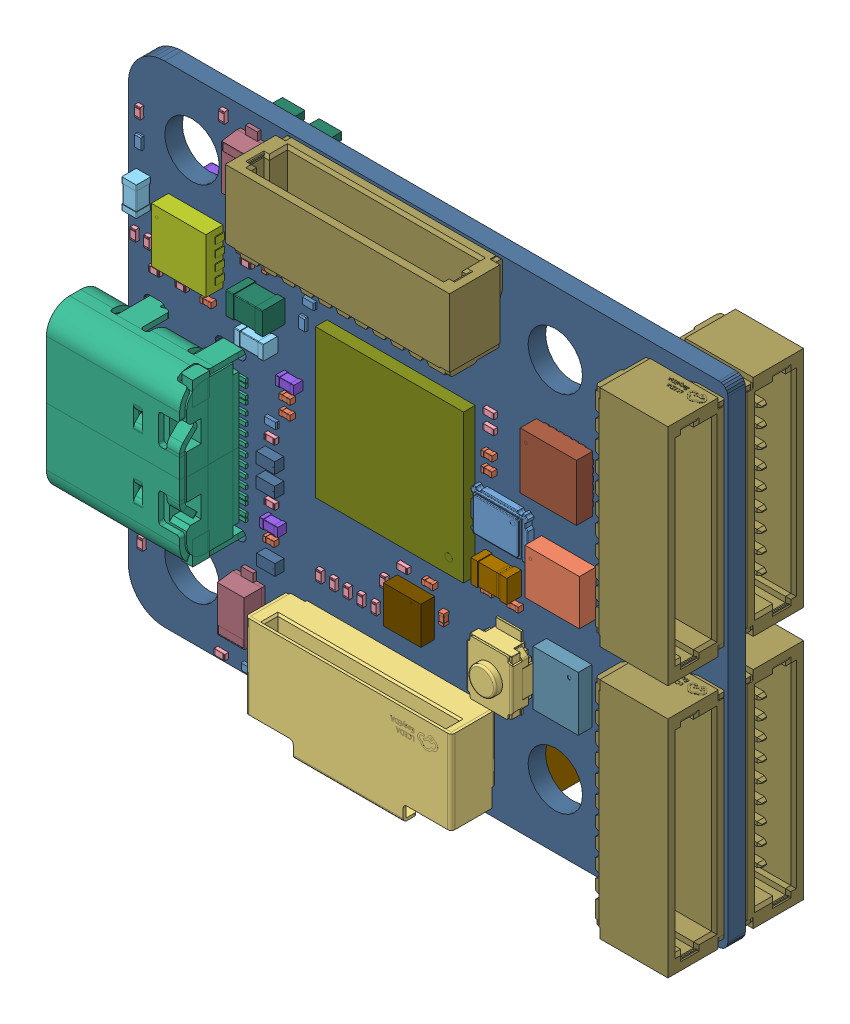
SolidWorks assembly NxtPX4, configuration 默认. Lengths in mm.
Overall size (34.16 27.21 7.57).
256 component instances, 28 part files, 0 mates.
Components (placement in the parent):
- NxtPX4.step-1: NxtPX4.step [默认] at origin size (34.16 27.21 7.57)
  - LED_0201_0603Metric.step-1: LED_0201_0603Metric.step [默认] at (3.0707 13.3273 1.012) x (-1 0 0) z (0 0 1) size (0.65 0.35 0.2)
    - SOLID.step-1: SOLID.step [默认] at origin size (0.65 0.35 0.2)
  - C_0201_0603Metric.step-1: C_0201_0603Metric.step [默认] at (-0.3793 17.3773 1.012) size (0.6 0.3 0.3)
    - SOLID-0.step-1: SOLID-0.step [默认] at origin size (0.6 0.3 0.3)
  - C_0201_0603Metric.step-2: C_0201_0603Metric.step [默认] at (15.0907 17.8073 1.012) size (0.6 0.3 0.3)
    - SOLID-0.step-1: SOLID-0.step [默认] at origin size (0.6 0.3 0.3)
  - C_0201_0603Metric.step-3: C_0201_0603Metric.step [默认] at (15.0707 11.3173 1.012) size (0.6 0.3 0.3)
    - SOLID-0.step-1: SOLID-0.step [默认] at origin size (0.6 0.3 0.3)
  - SW_SPST_B3U-1000P-B.step-1: SW_SPST_B3U-1000P-B.step [默认] at (16.1107 8.1973 1.012) x (0 1 0) z (0 0 1) size (4 2.51 2.09)
    - SOLID-1.step-1: SOLID-1.step [默认] at origin size (4 2.51 2.09)
  - R_0201_0603Metric.step-1: R_0201_0603Metric.step [默认] at (9.2907 8.8573 1.012) x (0 -1 0) z (0 0 1) size (0.6 0.3 0.23)
    - SOLID-2.step-1: SOLID-2.step [默认] at origin size (0.6 0.3 0.23)
  - LED_0201_0603Metric.step-2: LED_0201_0603Metric.step [默认] at (4.8107 18.9173 1.012) x (0 1 0) z (0 0 1) size (0.65 0.35 0.2)
    - SOLID.step-1: SOLID.step [默认] at origin size (0.65 0.35 0.2)
  - C_0603_1608Metric.step-1: C_0603_1608Metric.step [默认] at (2.5007 17.0773 1.012) size (1.6 0.8 0.8)
    - SOLID-3.step-1: SOLID-3.step [默认] at origin size (1.6 0.8 0.8)
  - USB_C_Receptacle_GCT_USB4105-xx-A_16P_TopMnt_Horizontal.step-1: USB_C_Receptacle_GCT_USB4105-xx-A_16P_TopMnt_Horizontal.step [默认] at (-2.4493 11.2373 1.012) x (0 -1 0) z (0 0 1) size (8.94 7.78 4.26)
    - COMPOUND.step-1: COMPOUND.step [默认] at origin size (8.94 7.78 4.26)
  - QFN8_3X3_MPS.step-1: QFN8_3X3_MPS.step [默认] at (-1.1693 19.8273 1.012) size (3.1 3 1)
    - COMPOUND-4.step-1: COMPOUND-4.step [默认] at origin size (3.1 3 1)
  - C_0603_1608Metric.step-2: C_0603_1608Metric.step [默认] at (-4.0893 20.7873 1.012) x (0 1 0) z (0 0 1) size (1.6 0.8 0.8)
    - SOLID-3.step-1: SOLID-3.step [默认] at origin size (1.6 0.8 0.8)
  - LED_0201_0603Metric.step-3: LED_0201_0603Metric.step [默认] at (5.1607 20.0473 1.012) size (0.65 0.35 0.2)
    - SOLID.step-1: SOLID.step [默认] at origin size (0.65 0.35 0.2)
  - R_0201_0603Metric.step-2: R_0201_0603Metric.step [默认] at (0.4307 26.6173 1.012) x (0 1 0) z (0 0 1) size (0.6 0.3 0.23)
    - SOLID-2.step-1: SOLID-2.step [默认] at origin size (0.6 0.3 0.23)
  - C_0402_1005Metric.step-1: C_0402_1005Metric.step [默认] at (4.1807 15.8173 1.012) x (-1 0 0) z (0 0 1) size (1 0.5 0.5)
    - SOLID-5.step-1: SOLID-5.step [默认] at origin size (1 0.5 0.5)
  - CAP_ABS07-32_768KHZ-T_ABR.step-1: CAP_ABS07-32_768KHZ-T_ABR.step [默认] at (15.7207 12.4073 1.012) x (-1 0 0) z (0 0 1) size (1.98 1.26 0.8)
    - COMPOUND-6.step-1: COMPOUND-6.step [默认] at origin size (1.98 1.26 0.8)
  - DFN1006-2_SOD882_NEX.step-1: DFN1006-2_SOD882_NEX.step [默认] at (3.1307 10.4373 1.012) x (-1 0 0) z (0 0 1) size (1.02 0.61 0.51)
    - COMPOUND-7.step-1: COMPOUND-7.step [默认] at origin size (1.02 0.61 0.51)
  - QFN24_3X3X0P9_IVS_ICM20649.step-1: QFN24_3X3X0P9_IVS_ICM20649.step [默认] at (19.1391 19.1673 1.012) size (3.1 3.1 0.94)
    - COMPOUND-8.step-1: COMPOUND-8.step [默认] at origin size (3.1 3.1 0.94)
  - C_0201_0603Metric.step-4: C_0201_0603Metric.step [默认] at (15.0807 17.0373 1.012) size (0.6 0.3 0.3)
    - SOLID-0.step-1: SOLID-0.step [默认] at origin size (0.6 0.3 0.3)
  - sh1.0_10P.step-1: sh1.0_10P.step [默认] at (9.7807 24.6273 1.012) x (-1 0 0) z (0 0 1) size (12.36 5 3.2)
    - COMPOUND-9.step-1: COMPOUND-9.step [默认] at origin size (12.36 5 3.2)
  - D_SOD-123F.step-1: D_SOD-123F.step [默认] at (2.0507 25.0998 1.012) x (0 -1 0) z (0 0 1) size (3.5 1.6 1.1)
    - SOLID-10.step-1: SOLID-10.step [默认] at origin size (3.5 1.6 1.1)
  - R_0201_0603Metric.step-3: R_0201_0603Metric.step [默认] at (-4.4593 18.5473 1.012) x (0 -1 0) z (0 0 1) size (0.6 0.3 0.23)
    - SOLID-2.step-1: SOLID-2.step [默认] at origin size (0.6 0.3 0.23)
  - LED_0201_0603Metric.step-4: LED_0201_0603Metric.step [默认] at (5.1607 20.8073 1.012) size (0.65 0.35 0.2)
    - SOLID.step-1: SOLID.step [默认] at origin size (0.65 0.35 0.2)
  - R_0201_0603Metric.step-4: R_0201_0603Metric.step [默认] at (3.0707 9.4673 1.012) x (-1 0 0) z (0 0 1) size (0.6 0.3 0.23)
    - SOLID-2.step-1: SOLID-2.step [默认] at origin size (0.6 0.3 0.23)
  - R_0201_0603Metric.step-5: R_0201_0603Metric.step [默认] at (-4.0793 4.0023 1.012) x (0 1 0) z (0 0 1) size (0.6 0.3 0.23)
    - SOLID-2.step-1: SOLID-2.step [默认] at origin size (0.6 0.3 0.23)
  - C_0201_0603Metric.step-5: C_0201_0603Metric.step [默认] at (3.9707 14.9473 1.012) x (-1 0 0) z (0 0 1) size (0.6 0.3 0.3)
    - SOLID-0.step-1: SOLID-0.step [默认] at origin size (0.6 0.3 0.3)
  - R_0201_0603Metric.step-6: R_0201_0603Metric.step [默认] at (5.7607 7.3673 1.012) x (0 1 0) z (0 0 1) size (0.6 0.3 0.23)
    - SOLID-2.step-1: SOLID-2.step [默认] at origin size (0.6 0.3 0.23)
  - LGA-14_3x2.5mm_P0.5mm_LayoutBorder3x4y.step-1: LGA-14_3x2.5mm_P0.5mm_LayoutBorder3x4y.step [默认] at (19.3757 8.9973 1.012) x (0 -1 0) z (0 0 1) size (3 2.5 0.78)
    - SOLID-11.step-1: SOLID-11.step [默认] at origin size (3 2.5 0.78)
  - R_0201_0603Metric.step-7: R_0201_0603Metric.step [默认] at (15.1207 19.0473 1.012) size (0.6 0.3 0.23)
    - SOLID-2.step-1: SOLID-2.step [默认] at origin size (0.6 0.3 0.23)
  - C_0805_2012Metric.step-1: C_0805_2012Metric.step [默认] at (2.7007 18.8773 1.012) size (2 1.25 1.25)
    - SOLID-12.step-1: SOLID-12.step [默认] at origin size (2 1.25 1.25)
  - C_0201_0603Metric.step-6: C_0201_0603Metric.step [默认] at (11.8257 10.0373 1.012) x (-1 0 0) z (0 0 1) size (0.6 0.3 0.3)
    - SOLID-0.step-1: SOLID-0.step [默认] at origin size (0.6 0.3 0.3)
  - R_0201_0603Metric.step-8: R_0201_0603Metric.step [默认] at (23.1807 13.9673 1.012) x (-1 0 0) z (0 0 1) size (0.6 0.3 0.23)
    - SOLID-2.step-1: SOLID-2.step [默认] at origin size (0.6 0.3 0.23)
  - C_0201_0603Metric.step-7: C_0201_0603Metric.step [默认] at (2.8507 20.6773 1.012) x (0 -1 0) z (0 0 1) size (0.6 0.3 0.3)
    - SOLID-0.step-1: SOLID-0.step [默认] at origin size (0.6 0.3 0.3)
  - R_0201_0603Metric.step-9: R_0201_0603Metric.step [默认] at (3.0707 12.5673 1.012) x (-1 0 0) z (0 0 1) size (0.6 0.3 0.23)
    - SOLID-2.step-1: SOLID-2.step [默认] at origin size (0.6 0.3 0.23)
  - sh1.0_10P.step-2: sh1.0_10P.step [默认] at (25.1807 20.9273 1.012) x (0 1 0) z (0 0 1) size (12.36 5 3.2)
    - COMPOUND-9.step-1: COMPOUND-9.step [默认] at origin size (12.36 5 3.2)
  - TFBGA100.step-1: TFBGA100.step [默认] at (10.0407 15.4873 0.512) x (-1 0 0) z (0 0 1) size (8.15 8.15 1.1)
    - COMPOUND-13.step-1: COMPOUND-13.step [默认] at origin size (8.15 8.15 1.1)
  - R_0201_0603Metric.step-10: R_0201_0603Metric.step [默认] at (15.1207 19.8073 1.012) x (-1 0 0) z (0 0 1) size (0.6 0.3 0.23)
    - SOLID-2.step-1: SOLID-2.step [默认] at origin size (0.6 0.3 0.23)
  - LED_0201_0603Metric.step-5: LED_0201_0603Metric.step [默认] at (-4.2093 23.0523 1.012) x (0 -1 0) z (0 0 1) size (0.65 0.35 0.2)
    - SOLID.step-1: SOLID.step [默认] at origin size (0.65 0.35 0.2)
  - R_0201_0603Metric.step-11: R_0201_0603Metric.step [默认] at (-3.6993 18.5473 1.012) x (0 -1 0) z (0 0 1) size (0.6 0.3 0.23)
    - SOLID-2.step-1: SOLID-2.step [默认] at origin size (0.6 0.3 0.23)
  - D_SOD-123F.step-2: D_SOD-123F.step [默认] at (1.8107 3.9373 1.012) x (0 1 0) z (0 0 1) size (3.5 1.6 1.1)
    - SOLID-10.step-1: SOLID-10.step [默认] at origin size (3.5 1.6 1.1)
  - D_SOD-523.step-1: D_SOD-523.step [默认] at (1.9607 22.1373 1.012) size (1.6 0.8 0.63)
    - SOLID-14.step-1: SOLID-14.step [默认] at origin size (1.6 0.8 0.63)
  - R_0201_0603Metric.step-12: R_0201_0603Metric.step [默认] at (8.8007 7.3673 1.012) x (0 1 0) z (0 0 1) size (0.6 0.3 0.23)
    - SOLID-2.step-1: SOLID-2.step [默认] at origin size (0.6 0.3 0.23)
  - sh1.0_10P.step-3: sh1.0_10P.step [默认] at (25.1807 6.9973 1.012) x (0 1 0) z (0 0 1) size (12.36 5 3.2)
    - COMPOUND-9.step-1: COMPOUND-9.step [默认] at origin size (12.36 5 3.2)
  - DFN1006-2_SOD882_NEX.step-2: DFN1006-2_SOD882_NEX.step [默认] at (3.1307 11.6073 1.012) x (-1 0 0) z (0 0 1) size (1.02 0.61 0.51)
    - COMPOUND-7.step-1: COMPOUND-7.step [默认] at origin size (1.02 0.61 0.51)
  - R_0201_0603Metric.step-13: R_0201_0603Metric.step [默认] at (-3.3093 17.3873 1.012) size (0.6 0.3 0.23)
    - SOLID-2.step-1: SOLID-2.step [默认] at origin size (0.6 0.3 0.23)
  - C_0201_0603Metric.step-8: C_0201_0603Metric.step [默认] at (3.0807 7.7273 1.012) size (0.6 0.3 0.3)
    - SOLID-0.step-1: SOLID-0.step [默认] at origin size (0.6 0.3 0.3)
  - C_0201_0603Metric.step-9: C_0201_0603Metric.step [默认] at (12.5807 8.7773 1.012) x (0 -1 0) z (0 0 1) size (0.6 0.3 0.3)
    - SOLID-0.step-1: SOLID-0.step [默认] at origin size (0.6 0.3 0.3)
  - QFN_BMP388_BOS.step-1: QFN_BMP388_BOS.step [默认] at (10.9607 8.4148 1.012) x (0 -1 0) z (0 0 1) size (2.06 2.06 0.82)
    - COMPOUND-15.step-1: COMPOUND-15.step [默认] at origin size (2.06 2.06 0.82)
  - R_0201_0603Metric.step-14: R_0201_0603Metric.step [默认] at (24.6607 13.9673 1.012) size (0.6 0.3 0.23)
    - SOLID-2.step-1: SOLID-2.step [默认] at origin size (0.6 0.3 0.23)
  - C_0402_1005Metric.step-2: C_0402_1005Metric.step [默认] at (3.2907 8.5973 1.012) size (1 0.5 0.5)
    - SOLID-5.step-1: SOLID-5.step [默认] at origin size (1 0.5 0.5)
  - R_0201_0603Metric.step-15: R_0201_0603Metric.step [默认] at (0.3157 0.9173 1.012) size (0.6 0.3 0.23)
    - SOLID-2.step-1: SOLID-2.step [默认] at origin size (0.6 0.3 0.23)
  - R_0201_0603Metric.step-16: R_0201_0603Metric.step [默认] at (8.0407 7.3673 1.012) x (0 1 0) z (0 0 1) size (0.6 0.3 0.23)
    - SOLID-2.step-1: SOLID-2.step [默认] at origin size (0.6 0.3 0.23)
  - Oscillator_SMD_Abracon_ASV-4Pin_7.0x5.1mm.step-1: Oscillator_SMD_Abracon_ASV-4Pin_7.0x5.1mm.step [默认] at (15.8307 14.9373 1.012) x (-1 0 0) z (0 0 1) size (3.15 2.29 0.55)
    - COMPOUND-16.step-1: COMPOUND-16.step [默认] at origin size (3.15 2.29 0.55)
  - R_0201_0603Metric.step-17: R_0201_0603Metric.step [默认] at (7.2807 7.3673 1.012) x (0 1 0) z (0 0 1) size (0.6 0.3 0.23)
    - SOLID-2.step-1: SOLID-2.step [默认] at origin size (0.6 0.3 0.23)
  - R_0201_0603Metric.step-18: R_0201_0603Metric.step [默认] at (1.7307 21.0273 1.012) size (0.6 0.3 0.23)
    - SOLID-2.step-1: SOLID-2.step [默认] at origin size (0.6 0.3 0.23)
  - R_0201_0603Metric.step-19: R_0201_0603Metric.step [默认] at (10.3607 10.0373 1.012) x (-1 0 0) z (0 0 1) size (0.6 0.3 0.23)
    - SOLID-2.step-1: SOLID-2.step [默认] at origin size (0.6 0.3 0.23)
  - LED_0201_0603Metric.step-6: LED_0201_0603Metric.step [默认] at (1.7907 0.9173 1.012) size (0.65 0.35 0.2)
    - SOLID.step-1: SOLID.step [默认] at origin size (0.65 0.35 0.2)
  - C_0201_0603Metric.step-10: C_0201_0603Metric.step [默认] at (3.9707 14.1873 1.012) x (-1 0 0) z (0 0 1) size (0.6 0.3 0.3)
    - SOLID-0.step-1: SOLID-0.step [默认] at origin size (0.6 0.3 0.3)
  - R_0201_0603Metric.step-20: R_0201_0603Metric.step [默认] at (1.7307 20.2673 1.012) x (-1 0 0) z (0 0 1) size (0.6 0.3 0.23)
    - SOLID-2.step-1: SOLID-2.step [默认] at origin size (0.6 0.3 0.23)
  - R_0201_0603Metric.step-21: R_0201_0603Metric.step [默认] at (-1.8493 17.3773 1.012) size (0.6 0.3 0.23)
    - SOLID-2.step-1: SOLID-2.step [默认] at origin size (0.6 0.3 0.23)
  - R_0201_0603Metric.step-22: R_0201_0603Metric.step [默认] at (-4.2093 24.5023 1.012) x (0 -1 0) z (0 0 1) size (0.6 0.3 0.23)
    - SOLID-2.step-1: SOLID-2.step [默认] at origin size (0.6 0.3 0.23)
  - LGA14_2P5X3X0P91_IVS_ICM42688-P.step-1: LGA14_2P5X3X0P91_IVS_ICM42688-P.step [默认] at (19.3707 14.0373 1.012) size (3 2.49 0.97)
    - COMPOUND-17.step-1: COMPOUND-17.step [默认] at origin size (3 2.49 0.97)
  - LED_0201_0603Metric.step-7: LED_0201_0603Metric.step [默认] at (-4.0793 5.4598 1.012) x (0 1 0) z (0 0 1) size (0.65 0.35 0.2)
    - SOLID.step-1: SOLID.step [默认] at origin size (0.65 0.35 0.2)
  - R_0201_0603Metric.step-23: R_0201_0603Metric.step [默认] at (6.5207 7.3673 1.012) x (0 1 0) z (0 0 1) size (0.6 0.3 0.23)
    - SOLID-2.step-1: SOLID-2.step [默认] at origin size (0.6 0.3 0.23)
  - C_0201_0603Metric.step-11: C_0201_0603Metric.step [默认] at (16.5307 11.3173 1.012) x (-1 0 0) z (0 0 1) size (0.6 0.3 0.3)
    - SOLID-0.step-1: SOLID-0.step [默认] at origin size (0.6 0.3 0.3)
  - sd_card.step-1: sd_card.step [默认] at (9.9307 2.6273 1.012) x (-1 0 0) z (0 0 1) size (11.35 5.5 2.5)
    - COMPOUND-18.step-1: COMPOUND-18.step [默认] at origin size (11.35 5.5 2.5)
  - R_0201_0603Metric.step-24: R_0201_0603Metric.step [默认] at (3.6407 20.8673 1.012) x (0 -1 0) z (0 0 1) size (0.6 0.3 0.23)
    - SOLID-2.step-1: SOLID-2.step [默认] at origin size (0.6 0.3 0.23)
  - DFN1006-2_SOD882_NEX.step-3: DFN1006-2_SOD882_NEX.step [默认] at (3.1507 6.7573 1.012) x (-1 0 0) z (0 0 1) size (1.02 0.61 0.51)
    - COMPOUND-7.step-1: COMPOUND-7.step [默认] at origin size (1.02 0.61 0.51)
  - C_0201_0603Metric.step-12: C_0201_0603Metric.step [默认] at (20.7107 13.7173 -0.05) x (0 -1 0) z (0 0 -1) size (0.6 0.3 0.3)
    - SOLID-0.step-1: SOLID-0.step [默认] at origin size (0.6 0.3 0.3)
  - C_0402_1005Metric.step-3: C_0402_1005Metric.step [默认] at (1.5707 14.1973 -0.05) x (-1 0 0) z (0 0 -1) size (1 0.5 0.5)
    - SOLID-5.step-1: SOLID-5.step [默认] at origin size (1 0.5 0.5)
  - D_SOD-123F.step-3: D_SOD-123F.step [默认] at (1.8207 3.8673 -0.05) x (0 1 0) z (0 0 -1) size (3.5 1.6 1.1)
    - SOLID-10.step-1: SOLID-10.step [默认] at origin size (3.5 1.6 1.1)
  - R_0201_0603Metric.step-25: R_0201_0603Metric.step [默认] at (12.6307 23.9173 -0.05) x (1 0 0) z (0 0 -1) size (0.6 0.3 0.23)
    - SOLID-2.step-1: SOLID-2.step [默认] at origin size (0.6 0.3 0.23)
  - R_0201_0603Metric.step-26: R_0201_0603Metric.step [默认] at (-0.7493 14.4773 -0.05) x (0 1 0) z (0 0 -1) size (0.6 0.3 0.23)
    - SOLID-2.step-1: SOLID-2.step [默认] at origin size (0.6 0.3 0.23)
  - C_0201_0603Metric.step-13: C_0201_0603Metric.step [默认] at (20.2007 9.1673 -0.05) x (0 -1 0) z (0 0 -1) size (0.6 0.3 0.3)
    - SOLID-0.step-1: SOLID-0.step [默认] at origin size (0.6 0.3 0.3)
  - C_0402_1005Metric.step-4: C_0402_1005Metric.step [默认] at (-1.6893 15.6973 -0.05) x (1 0 0) z (0 0 -1) size (1 0.5 0.5)
    - SOLID-5.step-1: SOLID-5.step [默认] at origin size (1 0.5 0.5)
  - C_0805_2012Metric.step-2: C_0805_2012Metric.step [默认] at (2.5907 19.0373 -0.05) x (1 0 0) z (0 0 -1) size (2 1.25 1.25)
    - SOLID-12.step-1: SOLID-12.step [默认] at origin size (2 1.25 1.25)
  - R_0201_0603Metric.step-27: R_0201_0603Metric.step [默认] at (-1.4193 8.7489 -0.05) x (0 1 0) z (0 0 -1) size (0.6 0.3 0.23)
    - SOLID-2.step-1: SOLID-2.step [默认] at origin size (0.6 0.3 0.23)
  - C_0201_0603Metric.step-14: C_0201_0603Metric.step [默认] at (8.0507 5.4373 -0.05) x (1 0 0) z (0 0 -1) size (0.6 0.3 0.3)
    - SOLID-0.step-1: SOLID-0.step [默认] at origin size (0.6 0.3 0.3)
  - R_0201_0603Metric.step-28: R_0201_0603Metric.step [默认] at (-4.0493 9.0773 -0.05) x (-1 0 0) z (0 0 -1) size (0.6 0.3 0.23)
    - SOLID-2.step-1: SOLID-2.step [默认] at origin size (0.6 0.3 0.23)
  - C_0402_1005Metric.step-5: C_0402_1005Metric.step [默认] at (8.2607 3.8073 -0.05) x (1 0 0) z (0 0 -1) size (1 0.5 0.5)
    - SOLID-5.step-1: SOLID-5.step [默认] at origin size (1 0.5 0.5)
  - C_0201_0603Metric.step-15: C_0201_0603Metric.step [默认] at (6.4507 12.7423 -0.05) x (0 1 0) z (0 0 -1) size (0.6 0.3 0.3)
    - SOLID-0.step-1: SOLID-0.step [默认] at origin size (0.6 0.3 0.3)
  - C_0402_1005Metric.step-6: C_0402_1005Metric.step [默认] at (1.3307 17.0873 -0.05) x (0 -1 0) z (0 0 -1) size (1 0.5 0.5)
    - SOLID-5.step-1: SOLID-5.step [默认] at origin size (1 0.5 0.5)
  - SOT-23.step-1: SOT-23.step [默认] at (11.4107 21.8173 -0.05) x (-1 0 0) z (0 0 -1) size (2.5 3 1.2)
    - SOLID-19.step-1: SOLID-19.step [默认] at origin size (2.5 3 1.2)
  - SOT-23.step-2: SOT-23.step [默认] at (2.5907 21.9973 -0.05) x (0 1 0) z (0 0 -1) size (2.5 3 1.2)
    - SOLID-19.step-1: SOLID-19.step [默认] at origin size (2.5 3 1.2)
  - C_0201_0603Metric.step-16: C_0201_0603Metric.step [默认] at (20.8007 18.5973 -0.05) x (0 -1 0) z (0 0 -1) size (0.6 0.3 0.3)
    - SOLID-0.step-1: SOLID-0.step [默认] at origin size (0.6 0.3 0.3)
  - C_0201_0603Metric.step-17: C_0201_0603Metric.step [默认] at (8.0507 4.6773 -0.05) x (1 0 0) z (0 0 -1) size (0.6 0.3 0.3)
    - SOLID-0.step-1: SOLID-0.step [默认] at origin size (0.6 0.3 0.3)
  - R_0402_1005Metric.step-1: R_0402_1005Metric.step [默认] at (-0.0993 21.3473 -0.05) x (-1 0 0) z (0 0 -1) size (1 0.5 0.35)
    - SOLID-20.step-1: SOLID-20.step [默认] at origin size (1 0.5 0.35)
  - R_0201_0603Metric.step-29: R_0201_0603Metric.step [默认] at (4.8107 18.9173 -0.05) x (0 1 0) z (0 0 -1) size (0.6 0.3 0.23)
    - SOLID-2.step-1: SOLID-2.step [默认] at origin size (0.6 0.3 0.23)
  - C_0201_0603Metric.step-18: C_0201_0603Metric.step [默认] at (15.9007 15.8573 -0.05) x (-1 0 0) z (0 0 -1) size (0.6 0.3 0.3)
    - SOLID-0.step-1: SOLID-0.step [默认] at origin size (0.6 0.3 0.3)
  - C_0402_1005Metric.step-7: C_0402_1005Metric.step [默认] at (12.3807 12.5373 -0.05) x (1 0 0) z (0 0 -1) size (1 0.5 0.5)
    - SOLID-5.step-1: SOLID-5.step [默认] at origin size (1 0.5 0.5)
  - SO-8_5.3x6.2mm_P1.27mm.step-1: SO-8_5.3x6.2mm_P1.27mm.step [默认] at (9.7107 9.1073 -0.05) x (-1 0 0) z (0 0 -1) size (8.4 6.2 1.6)
    - SOLID-21.step-1: SOLID-21.step [默认] at origin size (8.4 6.2 1.6)
  - R_0201_0603Metric.step-30: R_0201_0603Metric.step [默认] at (-1.7893 21.2273 -0.05) x (1 0 0) z (0 0 -1) size (0.6 0.3 0.23)
    - SOLID-2.step-1: SOLID-2.step [默认] at origin size (0.6 0.3 0.23)
  - R_0201_0603Metric.step-31: R_0201_0603Metric.step [默认] at (-2.1793 8.7389 -0.05) x (0 -1 0) z (0 0 -1) size (0.6 0.3 0.23)
    - SOLID-2.step-1: SOLID-2.step [默认] at origin size (0.6 0.3 0.23)
  - QFN8_3X3_MPS.step-2: QFN8_3X3_MPS.step [默认] at (-2.8293 11.5989 -0.05) x (0 1 0) z (0 0 -1) size (3.1 3 1)
    - COMPOUND-4.step-1: COMPOUND-4.step [默认] at origin size (3.1 3 1)
  - SOT-23-5_RIT.step-1: SOT-23-5_RIT.step [默认] at (5.1707 4.2573 -0.05) x (1 0 0) z (0 0 -1) size (3 3.13 1.72)
    - COMPOUND-22.step-1: COMPOUND-22.step [默认] at origin size (3 3.13 1.72)
  - C_0201_0603Metric.step-19: C_0201_0603Metric.step [默认] at (-2.9393 8.7389 -0.05) x (0 -1 0) z (0 0 -1) size (0.6 0.3 0.3)
    - SOLID-0.step-1: SOLID-0.step [默认] at origin size (0.6 0.3 0.3)
  - C_0201_0603Metric.step-20: C_0201_0603Metric.step [默认] at (15.5107 14.3373 -0.05) x (1 0 0) z (0 0 -1) size (0.6 0.3 0.3)
    - SOLID-0.step-1: SOLID-0.step [默认] at origin size (0.6 0.3 0.3)
  - C_0402_1005Metric.step-8: C_0402_1005Metric.step [默认] at (3.5007 1.7873 -0.05) x (0 -1 0) z (0 0 -1) size (1 0.5 0.5)
    - SOLID-5.step-1: SOLID-5.step [默认] at origin size (1 0.5 0.5)
  - C_0402_1005Metric.step-9: C_0402_1005Metric.step [默认] at (9.5907 15.1173 -0.05) x (-1 0 0) z (0 0 -1) size (1 0.5 0.5)
    - SOLID-5.step-1: SOLID-5.step [默认] at origin size (1 0.5 0.5)
  - C_0603_1608Metric.step-3: C_0603_1608Metric.step [默认] at (3.3207 6.8573 -0.05) x (1 0 0) z (0 0 -1) size (1.6 0.8 0.8)
    - SOLID-3.step-1: SOLID-3.step [默认] at origin size (1.6 0.8 0.8)
  - R_0201_0603Metric.step-32: R_0201_0603Metric.step [默认] at (4.4807 13.3223 -0.05) x (0 1 0) z (0 0 -1) size (0.6 0.3 0.23)
    - SOLID-2.step-1: SOLID-2.step [默认] at origin size (0.6 0.3 0.23)
  - L_Wuerth_MAPI-4030.step-1: L_Wuerth_MAPI-4030.step [默认] at (-1.7093 18.5673 -0.05) x (-1 0 0) z (0 0 -1) size (4.2 4 2.4)
    - SOLID-23.step-1: SOLID-23.step [默认] at origin size (4.2 4 2.4)
  - C_0201_0603Metric.step-21: C_0201_0603Metric.step [默认] at (18.9507 13.6573 -0.05) x (0 1 0) z (0 0 -1) size (0.6 0.3 0.3)
    - SOLID-0.step-1: SOLID-0.step [默认] at origin size (0.6 0.3 0.3)
  - C_0402_1005Metric.step-10: C_0402_1005Metric.step [默认] at (8.5307 16.0973 -0.05) x (-1 0 0) z (0 0 -1) size (1 0.5 0.5)
    - SOLID-5.step-1: SOLID-5.step [默认] at origin size (1 0.5 0.5)
  - C_0201_0603Metric.step-22: C_0201_0603Metric.step [默认] at (-3.2493 21.2273 -0.05) x (-1 0 0) z (0 0 -1) size (0.6 0.3 0.3)
    - SOLID-0.step-1: SOLID-0.step [默认] at origin size (0.6 0.3 0.3)
  - L_Wuerth_MAPI-4030.step-2: L_Wuerth_MAPI-4030.step [默认] at (1.5107 11.4373 -0.05) x (1 0 0) z (0 0 -1) size (4.2 4 2.4)
    - SOLID-23.step-1: SOLID-23.step [默认] at origin size (4.2 4 2.4)
  - C_0201_0603Metric.step-23: C_0201_0603Metric.step [默认] at (-4.0693 14.2373 -0.05) x (1 0 0) z (0 0 -1) size (0.6 0.3 0.3)
    - SOLID-0.step-1: SOLID-0.step [默认] at origin size (0.6 0.3 0.3)
  - R_0201_0603Metric.step-33: R_0201_0603Metric.step [默认] at (16.6207 9.3773 -0.05) x (0 1 0) z (0 0 -1) size (0.6 0.3 0.23)
    - SOLID-2.step-1: SOLID-2.step [默认] at origin size (0.6 0.3 0.23)
  - R_0201_0603Metric.step-34: R_0201_0603Metric.step [默认] at (-1.7693 7.6273 -0.05) x (-1 0 0) z (0 0 -1) size (0.6 0.3 0.23)
    - SOLID-2.step-1: SOLID-2.step [默认] at origin size (0.6 0.3 0.23)
  - C_0201_0603Metric.step-24: C_0201_0603Metric.step [默认] at (19.7207 17.4773 -0.05) x (1 0 0) z (0 0 -1) size (0.6 0.3 0.3)
    - SOLID-0.step-1: SOLID-0.step [默认] at origin size (0.6 0.3 0.3)
  - C_0201_0603Metric.step-25: C_0201_0603Metric.step [默认] at (20.9607 9.1673 -0.05) x (0 -1 0) z (0 0 -1) size (0.6 0.3 0.3)
    - SOLID-0.step-1: SOLID-0.step [默认] at origin size (0.6 0.3 0.3)
  - sh1.0_10P.step-4: sh1.0_10P.step [默认] at (25.1857 6.9973 -0.05) x (0 -1 0) z (0 0 -1) size (12.36 5 3.2)
    - COMPOUND-9.step-1: COMPOUND-9.step [默认] at origin size (12.36 5 3.2)
  - C_0201_0603Metric.step-26: C_0201_0603Metric.step [默认] at (8.4607 2.9273 -0.05) x (1 0 0) z (0 0 -1) size (0.6 0.3 0.3)
    - SOLID-0.step-1: SOLID-0.step [默认] at origin size (0.6 0.3 0.3)
  - R_0402_1005Metric.step-2: R_0402_1005Metric.step [默认] at (-2.3793 14.3673 -0.05) x (-1 0 0) z (0 0 -1) size (1 0.5 0.35)
    - SOLID-20.step-1: SOLID-20.step [默认] at origin size (1 0.5 0.35)
  - SOT-23.step-3: SOT-23.step [默认] at (18.4507 19.6173 -0.05) x (1 0 0) z (0 0 -1) size (2.5 3 1.2)
    - SOLID-19.step-1: SOLID-19.step [默认] at origin size (2.5 3 1.2)
  - C_0805_2012Metric.step-3: C_0805_2012Metric.step [默认] at (3.8907 25.6773 -0.05) x (0 1 0) z (0 0 -1) size (2 1.25 1.25)
    - SOLID-12.step-1: SOLID-12.step [默认] at origin size (2 1.25 1.25)
  - R_0201_0603Metric.step-35: R_0201_0603Metric.step [默认] at (5.1607 20.8073 -0.05) x (1 0 0) z (0 0 -1) size (0.6 0.3 0.23)
    - SOLID-2.step-1: SOLID-2.step [默认] at origin size (0.6 0.3 0.23)
  - C_0402_1005Metric.step-11: C_0402_1005Metric.step [默认] at (19.8407 13.8673 -0.05) x (0 -1 0) z (0 0 -1) size (1 0.5 0.5)
    - SOLID-5.step-1: SOLID-5.step [默认] at origin size (1 0.5 0.5)
  - C_0201_0603Metric.step-27: C_0201_0603Metric.step [默认] at (14.7907 15.4573 -0.05) x (0 1 0) z (0 0 -1) size (0.6 0.3 0.3)
    - SOLID-0.step-1: SOLID-0.step [默认] at origin size (0.6 0.3 0.3)
  - sh1.0_10P.step-5: sh1.0_10P.step [默认] at (25.1857 20.9273 -0.05) x (0 -1 0) z (0 0 -1) size (12.36 5 3.2)
    - COMPOUND-9.step-1: COMPOUND-9.step [默认] at origin size (12.36 5 3.2)
  - R_0201_0603Metric.step-36: R_0201_0603Metric.step [默认] at (10.8507 23.9173 -0.05) x (1 0 0) z (0 0 -1) size (0.6 0.3 0.23)
    - SOLID-2.step-1: SOLID-2.step [默认] at origin size (0.6 0.3 0.23)
  - C_0201_0603Metric.step-28: C_0201_0603Metric.step [默认] at (18.2607 17.4873 -0.05) x (1 0 0) z (0 0 -1) size (0.6 0.3 0.3)
    - SOLID-0.step-1: SOLID-0.step [默认] at origin size (0.6 0.3 0.3)
  - C_0805_2012Metric.step-4: C_0805_2012Metric.step [默认] at (1.8707 25.6773 -0.05) x (0 1 0) z (0 0 -1) size (2 1.25 1.25)
    - SOLID-12.step-1: SOLID-12.step [默认] at origin size (2 1.25 1.25)
  - R_0201_0603Metric.step-37: R_0201_0603Metric.step [默认] at (15.9007 15.0973 -0.05) x (-1 0 0) z (0 0 -1) size (0.6 0.3 0.23)
    - SOLID-2.step-1: SOLID-2.step [默认] at origin size (0.6 0.3 0.23)
  - sh1.0_4p.step-1: sh1.0_4p.step [默认] at (12.8107 3.2973 -0.05) x (-1 0 0) z (0 0 -1) size (6.4 5 3.2)
    - COMPOUND-24.step-1: COMPOUND-24.step [默认] at origin size (6.4 5 3.2)
  - SOT-23-5_RIT.step-2: SOT-23-5_RIT.step [默认] at (3.9507 16.2031 -0.05) x (1 0 0) z (0 0 -1) size (3 3.13 1.72)
    - COMPOUND-22.step-1: COMPOUND-22.step [默认] at origin size (3 3.13 1.72)
  - C_0603_1608Metric.step-4: C_0603_1608Metric.step [默认] at (3.3107 8.3873 -0.05) x (1 0 0) z (0 0 -1) size (1.6 0.8 0.8)
    - SOLID-3.step-1: SOLID-3.step [默认] at origin size (1.6 0.8 0.8)
  - R_0201_0603Metric.step-38: R_0201_0603Metric.step [默认] at (5.1607 20.0473 -0.05) x (1 0 0) z (0 0 -1) size (0.6 0.3 0.23)
    - SOLID-2.step-1: SOLID-2.step [默认] at origin size (0.6 0.3 0.23)
  - NxtPX4 PCB.step-1: NxtPX4 PCB.step [默认] at origin size (33 27 0.96)
